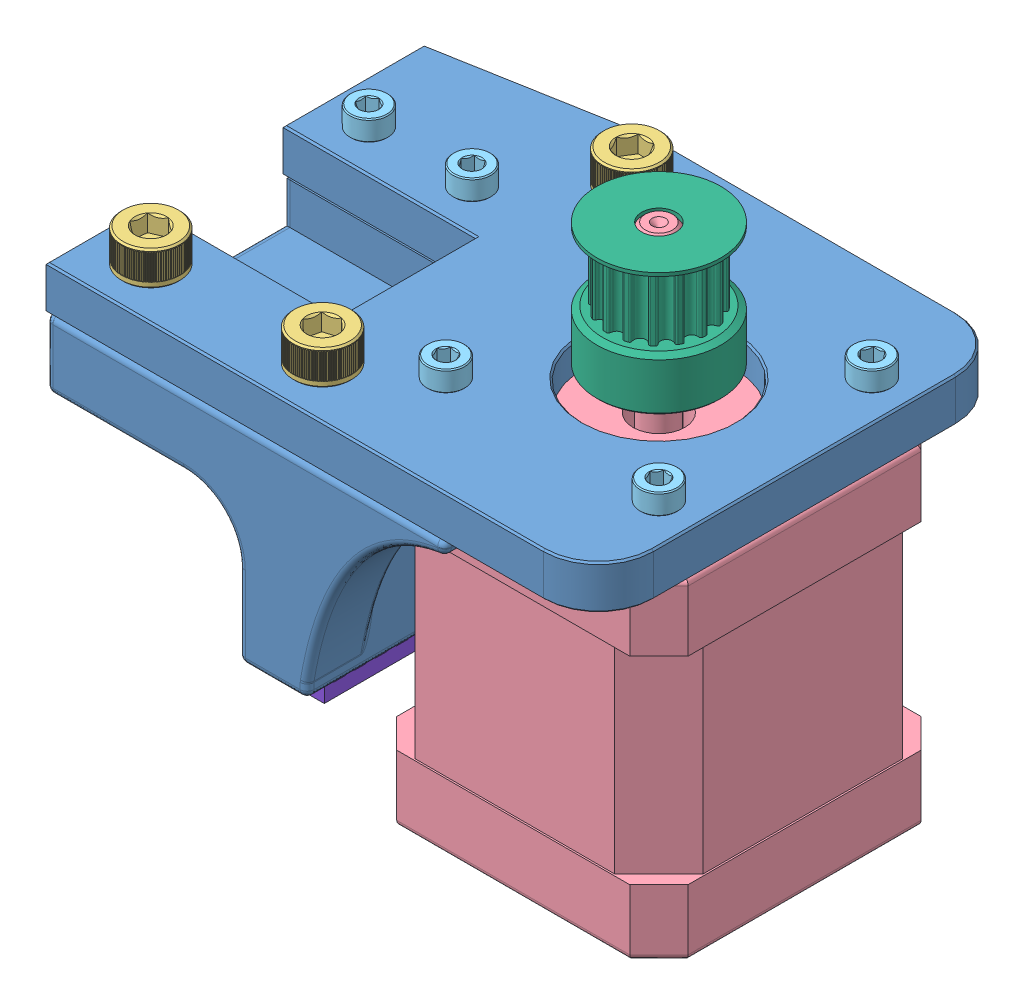
SolidWorks assembly x_motor_mount, configuration Default. Lengths in mm.
Overall size (80.4 74.04 62.99).
18 component instances, 8 part files, 36 mates.
Components (placement in the parent):
- v_rail_mount_x-1: v_rail_mount_x [Default] at (11.6499 65.9812 53.7622) size (80.4 38.16 62.99)
- 94180A361_Tapered Heat-Set Inserts for Plastic-2: 94180A361_Tapered Heat-Set Inserts for Plastic [94180A361] at (19.6499 72.6162 106.5122) x (0.881944 0 0.471354) z (0 1 0) size (8.33 8.33 7.05)
- 94180A361_Tapered Heat-Set Inserts for Plastic-3: 94180A361_Tapered Heat-Set Inserts for Plastic [94180A361] at (44.6499 72.6162 106.5122) x (0.881944 0 0.471354) z (0 1 0) size (8.33 8.33 7.05)
- 94180A361_Tapered Heat-Set Inserts for Plastic-4: 94180A361_Tapered Heat-Set Inserts for Plastic [94180A361] at (44.6499 72.6162 61.5122) x (0.881944 0 0.471354) z (0 1 0) size (8.33 8.33 7.05)
- 91290A231_Alloy Steel Socket Head Screw-2: 91290A231_Alloy Steel Socket Head Screw [91290A231] at (19.6499 77.3312 106.5122) x (0.395763 0 0.918353) z (0 1 0) size (8.5 8.5 20.34)
- 91290A231_Alloy Steel Socket Head Screw-3: 91290A231_Alloy Steel Socket Head Screw [91290A231] at (44.6499 77.3312 106.5122) x (0.293922 0 0.95583) z (0 1 0) size (8.5 8.5 20.34)
- 91290A231_Alloy Steel Socket Head Screw-4: 91290A231_Alloy Steel Socket Head Screw [91290A231] at (44.6499 77.3312 61.5122) x (-0.849967 0 -0.526836) z (0 1 0) size (8.5 8.5 20.34)
- 6627T91_Stepper Motor-1: 6627T91_Stepper Motor [6627T91] at (70.8499 64.9942 83.7622) x (1 0 0) z (0 1 0) size (42.4 43.16 74.04)
- 91290A572_Black-Oxide Alloy Steel Socket Head Screw-3: 91290A572_Black-Oxide Alloy Steel Socket Head Screw [15mm] at (86.3499 76.3312 68.2622) x (-0.782173 0 0.623061) z (0 1 0) size (5.5 5.5 18.14)
- 91290A572_Black-Oxide Alloy Steel Socket Head Screw-4: 91290A572_Black-Oxide Alloy Steel Socket Head Screw [15mm] at (55.3499 76.3312 68.2622) x (-0.819006 0 -0.573786) z (0 1 0) size (5.5 5.5 18.14)
- 91290A572_Black-Oxide Alloy Steel Socket Head Screw-5: 91290A572_Black-Oxide Alloy Steel Socket Head Screw [15mm] at (86.3499 76.3312 99.2622) x (-0.819006 0 -0.573786) z (0 1 0) size (5.5 5.5 18.14)
- 91290A572_Black-Oxide Alloy Steel Socket Head Screw-6: 91290A572_Black-Oxide Alloy Steel Socket Head Screw [15mm] at (55.3499 76.3312 99.2622) x (-0.819006 0 -0.573786) z (0 1 0) size (5.5 5.5 18.14)
- 3764N125_High-Strength Gt Timing Belt Pulley-1: 3764N125_High-Strength Gt Timing Belt Pulley [3764N125] at (70.8499 93.0132 83.7622) x (-0.993783 0 0.111333) z (0 -1 0) size (18.03 18.03 18)
- 91290A572_Black-Oxide Alloy Steel Socket Head Screw-8: 91290A572_Black-Oxide Alloy Steel Socket Head Screw [20mm] at (33.1499 73.8312 73.2622) x (-0.098871 0 -0.9951) z (0 1 0) size (5.5 5.5 23.14)
- 91290A572_Black-Oxide Alloy Steel Socket Head Screw-9: 91290A572_Black-Oxide Alloy Steel Socket Head Screw [20mm] at (18.1499 73.8312 73.2622) x (0.520474 0 -0.853877) z (0 1 0) size (5.5 5.5 23.14)
- 94180A331_Tapered Heat-Set Inserts for Plastic-6: 94180A331_Tapered Heat-Set Inserts for Plastic [94180A331] at (44.6499 47.8812 83.7622) x (0.757966 0 -0.652294) z (0 -1 0) size (5.56 5.56 3.99)
- belp_grip-2: belp_grip [Default] at (47.1499 41.9812 58.7622) x (0 0 1) z (-1 0 0) size (50 3.16 5)
- 91290A572_Black-Oxide Alloy Steel Socket Head Screw-13: 91290A572_Black-Oxide Alloy Steel Socket Head Screw [10] at (44.6499 45.4812 83.7622) x (-0.031298 0 0.99951) z (0 -1 0) size (5.5 5.5 13.14)
Mates (geometry in assembly coordinates):
- Concentric11: concentric aligned: cylinder of v_rail_mount_x-1 through (19.6499 67.9812 106.5122) axis (0 1 0) radius 4; cylinder of 94180A361_Tapered Heat-Set Inserts for Plastic-2 through (19.6499 75.9812 106.5122) axis (0 1 0) radius 4.165
- Coincident11: coincident aligned: plane of v_rail_mount_x-1 through (69.6499 75.9812 53.7622) normal (0 1 0); plane of 94180A361_Tapered Heat-Set Inserts for Plastic-2 through (20.8283 75.9812 104.3073) normal (0 1 0)
- Concentric21: concentric aligned: cylinder of v_rail_mount_x-1 through (44.6499 67.9812 106.5122) axis (0 1 0) radius 4; cylinder of 94180A361_Tapered Heat-Set Inserts for Plastic-3 through (44.6499 75.9812 106.5122) axis (0 1 0) radius 4.165
- Coincident21: coincident aligned: plane of v_rail_mount_x-1 through (69.6499 75.9812 53.7622) normal (0 1 0); plane of 94180A361_Tapered Heat-Set Inserts for Plastic-3 through (45.8283 75.9812 104.3073) normal (0 1 0)
- Concentric31: concentric aligned: cylinder of v_rail_mount_x-1 through (44.6499 67.9812 61.5122) axis (0 1 0) radius 4; cylinder of 94180A361_Tapered Heat-Set Inserts for Plastic-4 through (44.6499 75.9812 61.5122) axis (0 1 0) radius 4.165
- Coincident31: coincident aligned: plane of v_rail_mount_x-1 through (69.6499 75.9812 53.7622) normal (0 1 0); plane of 94180A361_Tapered Heat-Set Inserts for Plastic-4 through (45.8283 75.9812 59.3073) normal (0 1 0)
- Concentric41: concentric aligned: cone of v_rail_mount_x-1 through (19.6499 82.3312 106.5122) axis (0 -1 0); cone of 91290A231_Alloy Steel Socket Head Screw-2 through (19.6499 82.3312 106.5122) axis (0 -1 0)
- Coincident41: coincident anti-aligned: plane of v_rail_mount_x-1 through (11.6499 82.3312 53.7622) normal (0 1 0); plane of 91290A231_Alloy Steel Socket Head Screw-2 through (18.0669 82.3312 102.8388) normal (0 -1 0)
- Concentric51: concentric aligned: cone of v_rail_mount_x-1 through (44.6499 82.3312 106.5122) axis (0 -1 0); cone of 91290A231_Alloy Steel Socket Head Screw-3 through (44.6499 82.3312 106.5122) axis (0 -1 0)
- Coincident51: coincident anti-aligned: plane of v_rail_mount_x-1 through (11.6499 82.3312 53.7622) normal (0 1 0); plane of 91290A231_Alloy Steel Socket Head Screw-3 through (43.4742 82.3312 102.6889) normal (0 -1 0)
- Concentric61: concentric aligned: cone of v_rail_mount_x-1 through (44.6499 82.3312 61.5122) axis (0 -1 0); cone of 91290A231_Alloy Steel Socket Head Screw-4 through (44.6499 82.3312 61.5122) axis (0 -1 0)
- Coincident61: coincident anti-aligned: plane of v_rail_mount_x-1 through (11.6499 82.3312 53.7622) normal (0 1 0); plane of 91290A231_Alloy Steel Socket Head Screw-4 through (48.0498 82.3312 63.6195) normal (0 -1 0)
- Concentric7: concentric aligned: cylinder of v_rail_mount_x-1 through (70.8499 82.3312 83.7622) axis (0 -1 0) radius 11; cylinder of 6627T91_Stepper Motor-1 through (70.8499 78.0132 83.7622) axis (0 -1 0) radius 10.985
- Concentric8: concentric aligned: cylinder of v_rail_mount_x-1 through (86.3499 82.3312 99.2622) axis (0 -1 0) radius 1.5; circle of 6627T91_Stepper Motor-1
- Coincident7: coincident anti-aligned: plane of v_rail_mount_x-1 through (69.6499 75.9812 53.7622) normal (0 -1 0); plane of 6627T91_Stepper Motor-1 through (70.8499 75.9812 83.7622) normal (0 1 0)
- Concentric91: concentric aligned: cone of v_rail_mount_x-1 through (86.3499 82.0812 68.2622) axis (0 -1 0); cone of 91290A572_Black-Oxide Alloy Steel Socket Head Screw-3 through (86.3499 82.3312 68.2622) axis (0 -1 0)
- Coincident81: coincident anti-aligned: plane of v_rail_mount_x-1 through (11.6499 82.3312 53.7622) normal (0 1 0); plane of 91290A572_Black-Oxide Alloy Steel Socket Head Screw-3 through (87.9699 82.3312 70.2958) normal (0 -1 0)
- Concentric101: concentric aligned: cone of v_rail_mount_x-1 through (55.3499 82.0812 68.2622) axis (0 -1 0); cone of 91290A572_Black-Oxide Alloy Steel Socket Head Screw-4 through (55.3499 82.3312 68.2622) axis (0 -1 0)
- Coincident91: coincident anti-aligned: plane of v_rail_mount_x-1 through (11.6499 82.3312 53.7622) normal (0 1 0); plane of 91290A572_Black-Oxide Alloy Steel Socket Head Screw-4 through (53.8581 82.3312 70.3916) normal (0 -1 0)
- Concentric111: concentric aligned: cone of v_rail_mount_x-1 through (86.3499 82.0812 99.2622) axis (0 -1 0); cone of 91290A572_Black-Oxide Alloy Steel Socket Head Screw-5 through (86.3499 82.3312 99.2622) axis (0 -1 0)
- Coincident101: coincident anti-aligned: plane of v_rail_mount_x-1 through (11.6499 82.3312 53.7622) normal (0 1 0); plane of 91290A572_Black-Oxide Alloy Steel Socket Head Screw-5 through (84.8581 82.3312 101.3916) normal (0 -1 0)
- Concentric121: concentric aligned: cone of v_rail_mount_x-1 through (55.3499 82.0812 99.2622) axis (0 -1 0); cone of 91290A572_Black-Oxide Alloy Steel Socket Head Screw-6 through (55.3499 82.3312 99.2622) axis (0 -1 0)
- Coincident111: coincident anti-aligned: plane of v_rail_mount_x-1 through (11.6499 82.3312 53.7622) normal (0 1 0); plane of 91290A572_Black-Oxide Alloy Steel Socket Head Screw-6 through (53.8581 82.3312 101.3916) normal (0 -1 0)
- Concentric14: concentric aligned: cylinder of 6627T91_Stepper Motor-1 through (70.8499 102.0132 83.7622) axis (0 -1 0) radius 2.5; cylinder of 3764N125_High-Strength Gt Timing Belt Pulley-1 through (70.8499 84.0132 83.7622) axis (0 -1 0) radius 2.5
- Coincident13: coincident aligned: circle of 6627T91_Stepper Motor-1; plane of 3764N125_High-Strength Gt Timing Belt Pulley-1 through (71.8536 102.0132 92.7211) normal (0 1 0)
- Coincident141: coincident anti-aligned: plane of v_rail_mount_x-1 through (11.6499 82.3312 53.7622) normal (0 1 0); plane of 91290A572_Black-Oxide Alloy Steel Socket Head Screw-8 through (30.5626 82.3312 73.5192) normal (0 -1 0)
- Coincident151: coincident anti-aligned: plane of v_rail_mount_x-1 through (11.6499 82.3312 53.7622) normal (0 1 0); plane of 91290A572_Black-Oxide Alloy Steel Socket Head Screw-9 through (15.9298 82.3312 71.9089) normal (0 -1 0)
- Coincident17: coincident anti-aligned: circle of v_rail_mount_x-1; cylinder of 91290A572_Black-Oxide Alloy Steel Socket Head Screw-8 through (33.1499 62.3312 73.2622) axis (0 -1 0) radius 1.5
- Coincident18: coincident anti-aligned: circle of v_rail_mount_x-1; cylinder of 91290A572_Black-Oxide Alloy Steel Socket Head Screw-9 through (18.1499 62.3312 73.2622) axis (0 -1 0) radius 1.5
- Concentric201: concentric aligned: cylinder of v_rail_mount_x-1 through (44.6499 50.9812 83.7622) axis (0 -1 0) radius 2.5; cylinder of 94180A331_Tapered Heat-Set Inserts for Plastic-6 through (44.6499 45.9812 83.7622) axis (0 -1 0) radius 2.78
- Coincident221: coincident aligned: plane of v_rail_mount_x-1 through (49.6499 45.9812 113.7622) normal (0 -1 0); plane of 94180A331_Tapered Heat-Set Inserts for Plastic-6 through (45.6283 45.9812 84.8991) normal (0 -1 0)
- Concentric22: concentric anti-aligned: circle of 94180A331_Tapered Heat-Set Inserts for Plastic-6; cylinder of belp_grip-2 through (44.6499 38.9812 83.7622) axis (0 1 0) radius 1.5
- Distance1: distance = 2 mm anti-aligned: plane of belp_grip-2 through (42.1499 43.9812 58.7622) normal (0 1 0); plane of v_rail_mount_x-1 through (49.6499 45.9812 113.7622) normal (0 -1 0)
- Parallel4: parallel aligned: plane of v_rail_mount_x-1 through (39.6499 45.9812 113.7622) normal (-1 0 0); plane of belp_grip-2 through (42.1499 41.9812 58.7622) normal (-1 0 0)
- Concentric231: concentric aligned: cylinder of belp_grip-2 through (44.6499 38.9812 83.7622) axis (0 1 0) radius 1.5; cone of 91290A572_Black-Oxide Alloy Steel Socket Head Screw-13 through (44.6499 41.9812 83.7622) axis (0 1 0)
- Coincident271: coincident anti-aligned: plane of belp_grip-2 through (42.1499 41.9812 58.7622) normal (0 -1 0); plane of 91290A572_Black-Oxide Alloy Steel Socket Head Screw-13 through (42.0512 41.9812 83.6808) normal (0 1 0)
